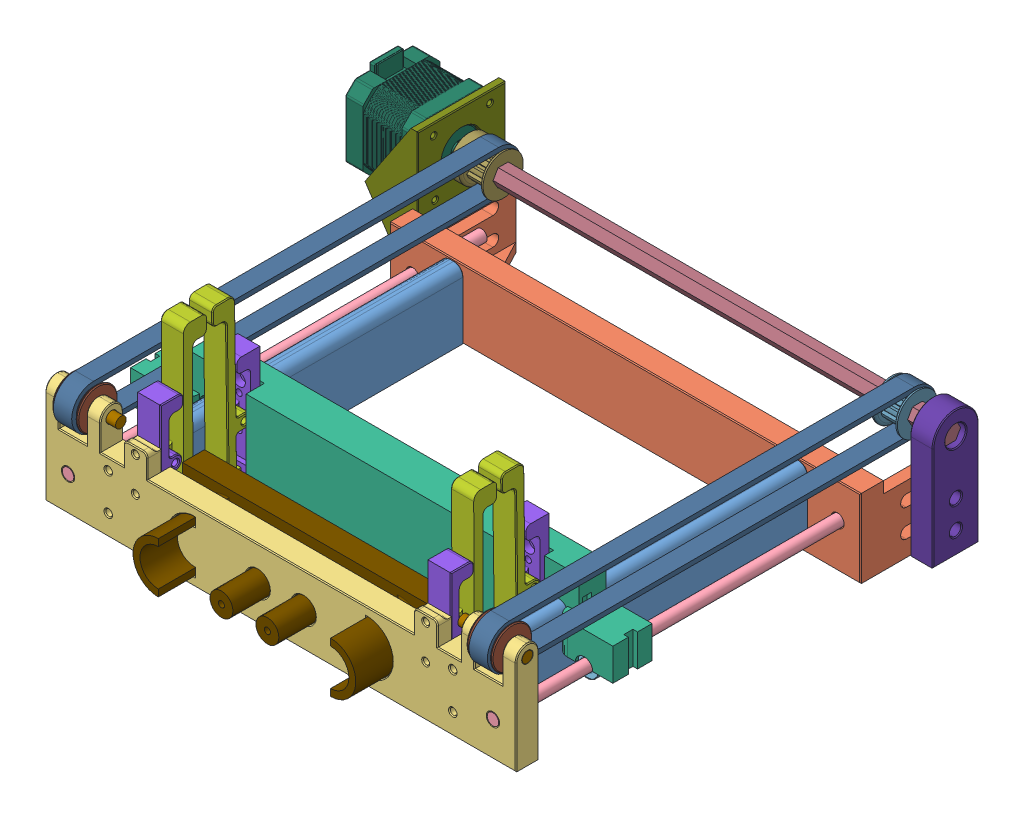
SolidWorks assembly Full Gantry Assembly, configuration Default. Lengths in mm.
Overall size (316.36 115.64 302.54).
38 component instances, 18 part files, 26 mates.
Components (placement in the parent):
- Gantry Frame Assembly-1: Gantry Frame Assembly [Default] at (-22.7812 29.2709 55.0882) size (260.35 63.5 254)
  - Frame Side Walls-1: Frame Side Walls [Default] at (-11.2932 98.0952 84.9503) size (12.1 37.5 177.8)
  - Gantry Frame End Piece-1: Gantry Frame End Piece [Default] at (83.9568 98.3952 72.2503) size (260.35 43.18 63.5)
  - Gantry Frame Heating End Piece-1: Gantry Frame Heating End Piece [Default] at (83.9568 98.3952 262.7503) size (260.35 58.42 12.7)
  - Frame Side Walls-2: Frame Side Walls [Default] at (179.2068 98.0952 84.9503) size (12.1 37.5 177.8)
  - 0.25 Diam 9 inch long Linear Rod-1: 0.25 Diam 9 inch long Linear Rod [Default] at (201.4318 98.3952 46.8503) x (0.968537 -0.248869 0) z (0 0 1) size (6.35 6.35 228.6)
  - 0.25 Diam 9 inch long Linear Rod-2: 0.25 Diam 9 inch long Linear Rod [Default] at (-33.5182 98.3952 46.8503) x (0.995745 -0.092157 0) z (0 0 1) size (6.35 6.35 228.6)
- Gantry Subassembly-1: Gantry Subassembly [Default] at (-16.8456 119.8156 304.6767) size (266.7 99.55 38.74)
  - 60595K11_Fixed Alignment Linear Ball Bearing-1: 60595K11_Fixed Alignment Linear Ball Bearing [60595K11] at (-39.4539 7.8505 -35.6605) size (12.7 12.7 19.05)
  - Gantry Piece-1: Gantry Piece [Default] at (78.0211 25.6305 -35.6605) size (266.7 50.8 22.23)
  - 60595K11_Fixed Alignment Linear Ball Bearing-2: 60595K11_Fixed Alignment Linear Ball Bearing [60595K11] at (195.4961 7.8505 -35.6605) x (0.99266 0.120939 0) z (0 0 1) size (12.7 12.7 19.05)
  - Clip Assembly-1: Clip Assembly [Default] at (45.7541 -13.0009 -33.2659) x (0 0.02134 0.999772) z (-1 0 0) size (28.26 95.92 12.7)
    - Added Clip Piece-1: Added Clip Piece [Default] at (13.6312 56.6752 41.3294) x (0.999405 -0.034486 0) z (0 0 1) size (20.96 95.25 12.7)
    - Attatched Clip Piece-1: Attatched Clip Piece [Default] at (0.3891 41.1725 54.0294) x (-0.999772 0.02134 0) z (0 0 -1) size (12.7 63.5 12.7)
  - Clip Assembly-2: Clip Assembly [Default] at (205.6471 -13.0009 -33.2659) x (0 0.02134 0.999772) z (-1 0 0) size (28.26 95.92 12.7)
    - Added Clip Piece-1: Added Clip Piece [Default] at (13.6312 56.6752 41.3294) x (0.999405 -0.034486 0) z (0 0 1) size (20.96 95.25 12.7)
    - Attatched Clip Piece-1: Attatched Clip Piece [Default] at (0.3891 41.1725 54.0294) x (-0.999772 0.02134 0) z (0 0 -1) size (12.7 63.5 12.7)
- Clip Assembly-1: Clip Assembly [Default] at (93.7601 105.5448 319.8889) x (0 0.02134 -0.999772) z (1 0 0) size (28.26 95.92 12.7) (flexible)
  - Added Clip Piece-1: Added Clip Piece [Default] at (13.4006 56.7842 41.3294) x (0.999804 -0.019788 0) z (0 0 1) size (20.96 95.25 12.7)
  - Attatched Clip Piece-1: Attatched Clip Piece [Default] at (0.3891 41.1725 54.0294) x (-0.999772 0.02134 0) z (0 0 -1) size (12.7 63.5 12.7)
- Clip Assembly-2: Clip Assembly [Default] at (-66.7679 105.5448 319.8889) x (0 0.02134 -0.999772) z (1 0 0) size (28.26 95.92 12.7) (flexible)
  - Added Clip Piece-1: Added Clip Piece [Default] at (13.4085 56.7805 41.3294) x (0.999794 -0.020292 0) z (0 0 1) size (20.96 95.25 12.7)
  - Attatched Clip Piece-1: Attatched Clip Piece [Default] at (0.3891 41.1725 54.0294) x (-0.999772 0.02134 0) z (0 0 -1) size (12.7 63.5 12.7)
- Passive Pulley Axle-1: Passive Pulley Axle [Default] at (-68.9995 160.6862 324.1885) x (0 -0.395908 -0.91829) z (0 -0.91829 0.395908) size (5.85 35.56 5.85)
- Passive Pulley Axle-2: Passive Pulley Axle [Default] at (191.3505 160.6862 324.1885) x (0 -0.802318 -0.596897) z (0 0.596897 -0.802318) size (5.85 35.56 5.85)
- Pulley and Belt Assembly-1: Pulley and Belt Assembly [Default] at (-262.393 22.4987 259.1542) x (0 0 -1) z (1 0 0) size (254.91 31.32 266.45) (flexible)
  - 20 Inch Belt-1: 20 Inch Belt [Default] at (47.0039 138.1875 203.6424) size (248.21 24.13 10.16)
  - Belt Idler Pulley-1: Belt Idler Pulley [6495K744] at (-65.0343 138.1875 212.2657) x (0.999956 -0.009357 0) z (0 0 1) size (22.23 22.23 14.3)
  - Belt Idler Pulley Coupler-1: Belt Idler Pulley Coupler [6495K744] at (159.0421 138.1875 205.9411) x (0.5 0.866025 0) z (0 0 -1) size (22.23 22.23 19.13)
  - Hexshaft Motor Drive Axle-1: Hexshaft Motor Drive Axle [Default] at (159.2153 138.1875 463.5733) x (0.5 -0.866025 0) z (0.866025 0.5 0) size (11 254 9.53)
  - Belt Idler Pulley Hex Hole-1: Belt Idler Pulley Hex Hole [6495K744] at (159.2153 138.1875 441.1959) x (-0.5 -0.866025 0) z (0 0 1) size (22.23 22.23 14.3)
  - Belt Idler Pulley-2: Belt Idler Pulley [6495K744] at (-64.8611 138.1875 441.1959) x (0.643871 0.765134 0) z (0 0 1) size (22.23 22.23 14.3)
  - 20 Inch Belt-2: 20 Inch Belt [Default] at (47.1771 138.1875 443.4946) x (1 0 0) z (0 0 -1) size (248.21 24.13 10.16)
- Stepper Mount and Tensioner-1: Stepper Mount and Tensioner [Default] at (-96.2784 207.8478 159.2914) x (1 0 0) z (0 -0.924225 0.381849) size (61.75 74.03 91.46)
  - Stepper Motor-1: Stepper Motor [Default] at (4.7189 -72.7035 20.9904) x (0 -0.924225 -0.381849) z (1 0 0) size (42.5 46.5 61.75)
  - Stepper Motor Mount-2: Stepper Motor Mount [Default] at (27.2789 -72.7035 20.9904) x (-1 0 0) z (0 -0.924225 -0.381849) size (29.21 76.08 48.66)
- Opposite tensioner-1: Opposite tensioner [Default] at (191.3505 103.5362 112.6389) x (0 0 -1) z (1 0 0) size (25.4 69.85 12.7)
- Spring Board-2: Spring Board [Default] at (-11.2145 108.6162 299.6968) x (1 0 0) z (0 -1 0) size (144.78 50.8 38.1)
Mates (geometry in assembly coordinates):
- Concentric1: concentric aligned: cylinder of Gantry Frame Assembly-1/0.25 Diam 9 inch long Linear Rod-2 through (-56.2995 127.6662 330.5385) axis (0 0 -1) radius 3.175; cylinder of Gantry Subassembly-1/60595K11_Fixed Alignment Linear Ball Bearing-1 through (-56.2995 127.6662 269.0162) axis (0 0 -1) radius 3.175
- Concentric2: concentric aligned: cylinder of Gantry Frame Assembly-1/0.25 Diam 9 inch long Linear Rod-1 through (178.6505 127.6662 330.5385) axis (0 0 -1) radius 3.175; cylinder of Gantry Subassembly-1/60595K11_Fixed Alignment Linear Ball Bearing-2 through (178.6505 127.6662 269.0162) axis (0 0 -1) radius 3.175
- Parallel1: parallel anti-aligned: plane of Gantry Frame Assembly-1/Frame Side Walls-2 through (150.3755 141.0362 317.8385) normal (-1 0 0); plane of Clip Assembly-1/Added Clip Piece-1 through (147.7895 118.7851 308.9051) normal (1 0 0)
- Concentric5: concentric aligned: cylinder of Gantry Frame Assembly-1/Gantry Frame Heating End Piece-1 through (141.4395 155.6062 330.5385) axis (0 0 -1) radius 1.7; cylinder of Clip Assembly-1/Attatched Clip Piece-1 through (141.4395 155.6062 338.1585) axis (0 0 -1) radius 1.7
- Parallel2: parallel anti-aligned: plane of Gantry Frame Assembly-1/Frame Side Walls-2 through (150.3755 141.0362 317.8385) normal (-1 0 0); plane of Clip Assembly-2/Added Clip Piece-1 through (-12.7385 118.7822 308.9192) normal (1 0 0)
- Concentric6: concentric aligned: cylinder of Gantry Frame Assembly-1/Gantry Frame Heating End Piece-1 through (-19.0885 155.6062 330.5385) axis (0 0 -1) radius 1.7; cylinder of Clip Assembly-2/Attatched Clip Piece-1 through (-19.0885 155.6062 338.1585) axis (0 0 -1) radius 1.7
- Concentric7: concentric anti-aligned: cylinder of Gantry Frame Assembly-1/Gantry Frame Heating End Piece-1 through (-134.0235 160.6862 324.1885) axis (1 0 0) radius 3.175; cylinder of Passive Pulley Axle-1 through (-33.4395 160.6862 324.1885) axis (-1 0 0) radius 2.925
- Coincident5: coincident aligned: plane of Gantry Frame Assembly-1/Gantry Frame Heating End Piece-1 through (-68.9995 146.7162 330.5385) normal (-1 0 0); plane of Passive Pulley Axle-1 through (-68.9995 160.6862 324.1885) normal (-1 0 0)
- Concentric10: concentric aligned: cylinder of Gantry Frame Assembly-1/Gantry Frame Heating End Piece-1 through (-134.0235 160.6862 324.1885) axis (1 0 0) radius 3.175; cylinder of Passive Pulley Axle-2 through (155.7905 160.6862 324.1885) axis (1 0 0) radius 2.925
- Coincident7: coincident aligned: plane of Gantry Frame Assembly-1/Gantry Frame Heating End Piece-1 through (191.3505 146.7162 330.5385) normal (1 0 0); plane of Passive Pulley Axle-2 through (191.3505 160.6862 324.1885) normal (1 0 0)
- Concentric11: concentric anti-aligned: cylinder of Passive Pulley Axle-1 through (-33.4395 160.6862 324.1885) axis (-1 0 0) radius 2.925; cylinder of Pulley and Belt Assembly-1/Belt Idler Pulley-1 through (-39.8149 160.6862 324.1885) axis (1 0 0) radius 3.175
- Coincident8: coincident anti-aligned: plane of Gantry Frame Assembly-1/Gantry Frame Heating End Piece-1 through (-46.1395 167.0362 330.5385) normal (-1 0 0); plane of Pulley and Belt Assembly-1/Belt Idler Pulley-1 through (-46.1395 157.5113 324.2182) normal (1 0 0)
- Parallel3: parallel aligned: plane of Gantry Subassembly-1/Gantry Piece-1 through (-46.7745 145.4462 259.4912) normal (0 1 0); plane of Pulley and Belt Assembly-1/20 Inch Belt-1 through (-48.5906 172.7512 324.1885) normal (0 1 0)
- Coincident10: coincident anti-aligned: plane of Gantry Frame Assembly-1/Gantry Frame Heating End Piece-1 through (168.4905 167.0362 330.5385) normal (1 0 0); plane of Pulley and Belt Assembly-1/Belt Idler Pulley-2 through (168.4905 153.5312 315.5127) normal (-1 0 0)
- Parallel9: parallel aligned: plane of Gantry Frame Assembly-1/Gantry Frame End Piece-1 through (61.1755 103.5362 127.3385) normal (0 -1 0); plane of Stepper Mount and Tensioner-1/Stepper Motor Mount-2 through (-72.8095 105.8113 121.9021) normal (0 -1 0)
- Slot1: slot aligned: cylinder of Stepper Mount and Tensioner-1/Stepper Motor Mount-2 through (-72.8095 130.8412 100.1121) axis (1 0 0) radius 3.175; plane of Gantry Frame Assembly-1/Gantry Frame End Piece-1 through (-113.4495 127.6662 89.2385) normal (0 1 0); cylinder of Gantry Frame Assembly-1/Gantry Frame End Piece-1 through (-113.4495 130.8412 114.6385) axis (1 0 0) radius 3.175
- Slot2: slot aligned: cylinder of Stepper Mount and Tensioner-1/Stepper Motor Mount-2 through (-72.8095 115.6012 100.1121) axis (1 0 0) radius 3.175; plane of Gantry Frame Assembly-1/Gantry Frame End Piece-1 through (-113.4495 112.4262 89.2385) normal (0 1 0); cylinder of Gantry Frame Assembly-1/Gantry Frame End Piece-1 through (-113.4495 115.6012 114.6385) axis (1 0 0) radius 3.175
- Coincident18: coincident anti-aligned: plane of Gantry Frame Assembly-1/Gantry Frame End Piece-1 through (-68.9995 146.7162 140.0385) normal (-1 0 0); plane of Stepper Mount and Tensioner-1/Stepper Motor Mount-2 through (-68.9995 160.6862 100.1121) normal (1 0 0)
- Coincident19: coincident anti-aligned: plane of Gantry Frame Assembly-1/Gantry Frame End Piece-1 through (191.3505 146.7162 140.0385) normal (1 0 0); plane of Opposite tensioner-1 through (191.3505 160.6862 99.9389) normal (-1 0 0)
- Slot3: slot aligned: plane of Gantry Frame Assembly-1/Gantry Frame End Piece-1 through (235.8005 127.6662 89.2385) normal (0 1 0); cylinder of Opposite tensioner-1 through (204.0505 130.8412 99.9389) axis (-1 0 0) radius 3.175; cylinder of Gantry Frame Assembly-1/Gantry Frame End Piece-1 through (235.8005 130.8412 89.2385) axis (-1 0 0) radius 3.175
- Slot4: slot aligned: plane of Gantry Frame Assembly-1/Gantry Frame End Piece-1 through (235.8005 112.4262 89.2385) normal (0 1 0); cylinder of Opposite tensioner-1 through (204.0505 115.6012 99.9389) axis (-1 0 0) radius 3.175; cylinder of Gantry Frame Assembly-1/Gantry Frame End Piece-1 through (235.8005 115.6012 89.2385) axis (-1 0 0) radius 3.175
- Concentric12: concentric: cylinder of Pulley and Belt Assembly-1/Belt Idler Pulley Coupler-1 through (-66.7643 160.6862 100.1121) axis (-1 0 0) radius 2.5; cylinder of Stepper Mount and Tensioner-1/Stepper Motor-1 through (-50.5595 160.6862 100.1121) axis (-1 0 0) radius 2.5
- Concentric15: concentric anti-aligned: cylinder of Pulley and Belt Assembly-1/Belt Idler Pulley Hex Hole-1 through (189.1153 160.6862 99.9389) axis (1 0 0) radius 11.1125; cylinder of Opposite tensioner-1 through (204.0505 160.6862 99.9389) axis (-1 0 0) radius 5.715
- Concentric16: concentric anti-aligned: cylinder of Gantry Frame Assembly-1/Gantry Frame Heating End Piece-1 through (48.4755 127.6662 317.8385) axis (0 0 1) radius 6.6; cylinder of Spring Board-2 through (48.4755 127.6662 350.4968) axis (0 0 -1) radius 6.35
- Concentric17: concentric anti-aligned: cylinder of Gantry Frame Assembly-1/Gantry Frame Heating End Piece-1 through (73.8755 127.6662 317.8385) axis (0 0 1) radius 6.6; cylinder of Spring Board-2 through (73.8755 127.6662 350.4968) axis (0 0 -1) radius 6.35
- Coincident21: coincident anti-aligned: plane of Gantry Frame Assembly-1/Gantry Frame Heating End Piece-1 through (145.5035 156.8762 322.9185) normal (0 0 -1); plane of Clip Assembly-1/Attatched Clip Piece-1 through (135.0895 178.4662 322.9185) normal (0 0 1)
